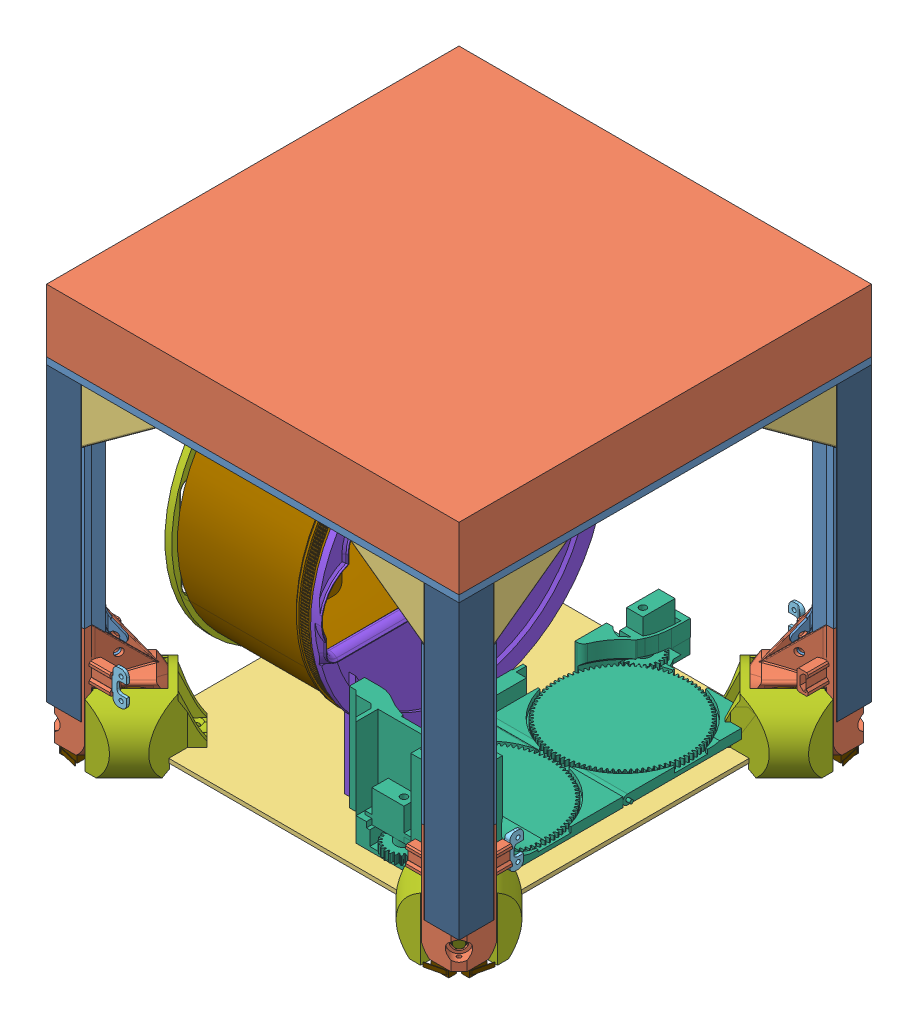
SolidWorks assembly MK7 IEEE BOT, configuration Default. Lengths in mm.
Overall size (425.24 302.29 425.24).
113 component instances, 29 part files, 44 mates.
Components (placement in the parent):
- MK5 Top Plate-1: MK5 Top Plate [Default] at (0 249 0) size (301.62 5 301.62)
- LEG assem MK5-1: LEG assem MK5 [Default] at (121.6905 25.4 121.6905) x (-0.707107 0 0.707107) z (-0.707107 0 -0.707107) size (113.86 301.29 113.86)
  - Omniwheel Mount-MK5-1: Omniwheel Mount-MK5 [Default] x (0 0 -1) z (1 0 0) size (67.69 82.93 55.08)
  - Leg Bracket MK5-1: Leg Bracket MK5 [Default] at (0 223.6 -41.1848) x (-0.707107 0 0.707107) z (-0.707107 0 -0.707107) size (80.51 40 80.51)
  - Omniwheel Hub-1: Omniwheel Hub [Default] at (0 0 13.95) x (-0.608761 -0.793353 0) z (0.793353 -0.608761 0) size (15.82 24.5 15.7)
  - TOF sensor mount-1: TOF sensor mount [Default] at (-9.5304 0 9.5304) x (0.707107 0 0.707107) z (-0.707107 0 0.707107) size (3.8 25 24.25)
  - Pinion Drive-1: Pinion Drive [Default] at (-0.7071 228.6 -26.6539) size (107.48 45 51.62)
  - Bottom Plate Bracket-1: Bottom Plate Bracket [Default] at (0 0 21.75) size (66.29 52.5 63.07)
  - Bearing Slider-1: Bearing Slider [Default] at (-0.7071 261.6 -26.6539) x (1 0 0) z (0 1 0) size (23.6 12.46 20)
  - 2in 14mm omniwheel-MK5-1: 2in 14mm omniwheel-MK5 [Default] at origin size (55.39 55.39 27.5)
  - Steel 90 degree MK5-1: Steel 90 degree MK5 [8982K151] at (0 120.65 -23.2243) x (-0.707107 0 -0.707107) z (0 1 0) size (25.4 25.4 213.6)
  - Nema17.step-2: Nema17.step [Default] at (22.8737 252.6 18.2122) x (0 -1 0) z (-1 0 0) size (42 57.7 46)
  - hex flange nut_am-2: hex flange nut_am [B18.2.2.4M - Hex flange nut, M6 x 1 --N] at (0 0 27.75) x (0.990831 -0.135106 0) z (0 0 1) size (14.2 14.2 6)
  - instrument ball bearing_68_am-4: instrument ball bearing_68_am [AFBMA 12.1.4.1 - 0070-14 - 12,SI,NC,12_68] at (0 0 -22.7198) x (0 0 1) z (-0.999767 0.021607 0) size (3.5 14 14)
  - 6mm G2T Pully Gear-1: 6mm G2T Pully Gear [Default] at (0 0 -9.25) x (0.996082 -0.088439 0) z (0.088439 0.996082 0) size (16 16 16)
  - 6mm G2T Pully Gear-2: 6mm G2T Pully Gear [Default] at (0 249.6 -30.45) x (-0.989152 0.146897 0) z (0.146897 0.989152 0) size (16 16 16)
  - Belt-1: Belt [Default] at (0 249.6 -23.35) x (-0.989152 0.146897 0) z (0 0 1) size (51.67 261.89 6)
  - instrument ball bearing_68_am-5: instrument ball bearing_68_am [AFBMA 12.1.4.1 - 0070-14 - 12,SI,NC,12_68] at (0 0 20) x (0 0 1) z (-0.999898 0.014309 0) size (3.5 14 14)
  - hex flange screw_am-1: hex flange screw_am [B18.2.3.4M - Hex flange screw, M5 x 0.8 x 35 --16N] at (0 0 -30.0698) x (0 0 1) z (-0.776229 0.630451 0) size (40.6 11.4 11.4)
  - hex flange screw_am-2: hex flange screw_am [B18.2.3.4M - Hex flange screw, M5 x 0.8 x 35 --16N] at (0 249.6 10.15) x (0 0 -1) z (-0.786653 -0.617395 0) size (40.6 11.4 11.4)
  - instrument ball bearing_68_am-6: instrument ball bearing_68_am [AFBMA 12.1.4.1 - 0070-14 - 12,SI,NC,12_68] at (0 251.6 -10.2) x (0 0 1) z (-0.998037 -0.06263 0) size (3.5 14 14)
  - instrument ball bearing_68_am-7: instrument ball bearing_68_am [AFBMA 12.1.4.1 - 0070-14 - 12,SI,NC,12_68] at (0 251.6 -2.2359) x (0 0 1) z (-0.682316 -0.731058 0) size (3.5 14 14)
  - hex screw_am-1: hex screw_am [B18.6.7M - M4 x 0.7 x 40 Indented HHMS --40N] at (5 274.6 -7.2179) x (0 -1 0) z (0 0 1) size (43 8.08 7)
  - Microswitch-1: Microswitch [Default] at (5.7276 -18.7296 -25.8406) x (0.707107 0 0.707107) z (-0.707107 0 0.707107) size (15.16 5.8 14.13)
  - Microswitch-2: Microswitch [Default] at (-5.7276 -12.9296 -25.8406) x (-0.707107 0 0.707107) z (0.707107 0 0.707107) size (15.16 5.8 14.13)
  - BeltShroud-1: BeltShroud [Default] at (0 70 0) x (0 0 -1) z (0 1 0) size (24.44 39.03 180.07)
- LEG assem MK5-2: LEG assem MK5 [Default] at (121.6905 25.4 -121.6905) x (0.707107 0 0.707107) z (-0.707107 0 0.707107) size (113.86 301.29 113.86)
  - Omniwheel Mount-MK5-1: Omniwheel Mount-MK5 [Default] x (0 0 -1) z (1 0 0) size (67.69 82.93 55.08)
  - Leg Bracket MK5-1: Leg Bracket MK5 [Default] at (0 223.6 -41.1848) x (-0.707107 0 0.707107) z (-0.707107 0 -0.707107) size (80.51 40 80.51)
  - Omniwheel Hub-1: Omniwheel Hub [Default] at (0 0 13.95) x (-0.608761 -0.793353 0) z (0.793353 -0.608761 0) size (15.82 24.5 15.7)
  - TOF sensor mount-1: TOF sensor mount [Default] at (-9.5304 0 9.5304) x (0.707107 0 0.707107) z (-0.707107 0 0.707107) size (3.8 25 24.25)
  - Pinion Drive-1: Pinion Drive [Default] at (-0.7071 228.6 -26.6539) size (107.48 45 51.62)
  - Bottom Plate Bracket-1: Bottom Plate Bracket [Default] at (0 0 21.75) size (66.29 52.5 63.07)
  - Bearing Slider-1: Bearing Slider [Default] at (-0.7071 261.6 -26.6539) x (1 0 0) z (0 1 0) size (23.6 12.46 20)
  - 2in 14mm omniwheel-MK5-1: 2in 14mm omniwheel-MK5 [Default] at origin size (55.39 55.39 27.5)
  - Steel 90 degree MK5-1: Steel 90 degree MK5 [8982K151] at (0 120.65 -23.2243) x (-0.707107 0 -0.707107) z (0 1 0) size (25.4 25.4 213.6)
  - Nema17.step-2: Nema17.step [Default] at (22.8737 252.6 18.2122) x (0 -1 0) z (-1 0 0) size (42 57.7 46)
  - hex flange nut_am-2: hex flange nut_am [B18.2.2.4M - Hex flange nut, M6 x 1 --N] at (0 0 27.75) x (0.990831 -0.135106 0) z (0 0 1) size (14.2 14.2 6)
  - instrument ball bearing_68_am-4: instrument ball bearing_68_am [AFBMA 12.1.4.1 - 0070-14 - 12,SI,NC,12_68] at (0 0 -22.7198) x (0 0 1) z (-0.999767 0.021607 0) size (3.5 14 14)
  - 6mm G2T Pully Gear-1: 6mm G2T Pully Gear [Default] at (0 0 -9.25) x (0.996082 -0.088439 0) z (0.088439 0.996082 0) size (16 16 16)
  - 6mm G2T Pully Gear-2: 6mm G2T Pully Gear [Default] at (0 249.6 -30.45) x (-0.989152 0.146897 0) z (0.146897 0.989152 0) size (16 16 16)
  - Belt-1: Belt [Default] at (0 249.6 -23.35) x (-0.989152 0.146897 0) z (0 0 1) size (51.67 261.89 6)
  - instrument ball bearing_68_am-5: instrument ball bearing_68_am [AFBMA 12.1.4.1 - 0070-14 - 12,SI,NC,12_68] at (0 0 20) x (0 0 1) z (-0.999898 0.014309 0) size (3.5 14 14)
  - hex flange screw_am-1: hex flange screw_am [B18.2.3.4M - Hex flange screw, M5 x 0.8 x 35 --16N] at (0 0 -30.0698) x (0 0 1) z (-0.776229 0.630451 0) size (40.6 11.4 11.4)
  - hex flange screw_am-2: hex flange screw_am [B18.2.3.4M - Hex flange screw, M5 x 0.8 x 35 --16N] at (0 249.6 10.15) x (0 0 -1) z (-0.786653 -0.617395 0) size (40.6 11.4 11.4)
  - instrument ball bearing_68_am-6: instrument ball bearing_68_am [AFBMA 12.1.4.1 - 0070-14 - 12,SI,NC,12_68] at (0 251.6 -10.2) x (0 0 1) z (-0.998037 -0.06263 0) size (3.5 14 14)
  - instrument ball bearing_68_am-7: instrument ball bearing_68_am [AFBMA 12.1.4.1 - 0070-14 - 12,SI,NC,12_68] at (0 251.6 -2.2359) x (0 0 1) z (-0.682316 -0.731058 0) size (3.5 14 14)
  - hex screw_am-1: hex screw_am [B18.6.7M - M4 x 0.7 x 40 Indented HHMS --40N] at (5 274.6 -7.2179) x (0 -1 0) z (0 0 1) size (43 8.08 7)
  - Microswitch-1: Microswitch [Default] at (5.7276 -18.7296 -25.8406) x (0.707107 0 0.707107) z (-0.707107 0 0.707107) size (15.16 5.8 14.13)
  - Microswitch-2: Microswitch [Default] at (-5.7276 -12.9296 -25.8406) x (-0.707107 0 0.707107) z (0.707107 0 0.707107) size (15.16 5.8 14.13)
  - BeltShroud-1: BeltShroud [Default] at (0 70 0) x (0 0 -1) z (0 1 0) size (24.44 39.03 180.07)
- LEG assem MK5-3: LEG assem MK5 [Default] at (-121.6905 25.4 -121.6905) x (0.707107 0 -0.707107) z (0.707107 0 0.707107) size (113.86 301.29 113.86)
  - Omniwheel Mount-MK5-1: Omniwheel Mount-MK5 [Default] x (0 0 -1) z (1 0 0) size (67.69 82.93 55.08)
  - Leg Bracket MK5-1: Leg Bracket MK5 [Default] at (0 223.6 -41.1848) x (-0.707107 0 0.707107) z (-0.707107 0 -0.707107) size (80.51 40 80.51)
  - Omniwheel Hub-1: Omniwheel Hub [Default] at (0 0 13.95) x (-0.608761 -0.793353 0) z (0.793353 -0.608761 0) size (15.82 24.5 15.7)
  - TOF sensor mount-1: TOF sensor mount [Default] at (-9.5304 0 9.5304) x (0.707107 0 0.707107) z (-0.707107 0 0.707107) size (3.8 25 24.25)
  - Pinion Drive-1: Pinion Drive [Default] at (-0.7071 228.6 -26.6539) size (107.48 45 51.62)
  - Bottom Plate Bracket-1: Bottom Plate Bracket [Default] at (0 0 21.75) size (66.29 52.5 63.07)
  - Bearing Slider-1: Bearing Slider [Default] at (-0.7071 261.6 -26.6539) x (1 0 0) z (0 1 0) size (23.6 12.46 20)
  - 2in 14mm omniwheel-MK5-1: 2in 14mm omniwheel-MK5 [Default] at origin size (55.39 55.39 27.5)
  - Steel 90 degree MK5-1: Steel 90 degree MK5 [8982K151] at (0 120.65 -23.2243) x (-0.707107 0 -0.707107) z (0 1 0) size (25.4 25.4 213.6)
  - Nema17.step-2: Nema17.step [Default] at (22.8737 252.6 18.2122) x (0 -1 0) z (-1 0 0) size (42 57.7 46)
  - hex flange nut_am-2: hex flange nut_am [B18.2.2.4M - Hex flange nut, M6 x 1 --N] at (0 0 27.75) x (0.990831 -0.135106 0) z (0 0 1) size (14.2 14.2 6)
  - instrument ball bearing_68_am-4: instrument ball bearing_68_am [AFBMA 12.1.4.1 - 0070-14 - 12,SI,NC,12_68] at (0 0 -22.7198) x (0 0 1) z (-0.999767 0.021607 0) size (3.5 14 14)
  - 6mm G2T Pully Gear-1: 6mm G2T Pully Gear [Default] at (0 0 -9.25) x (0.996082 -0.088439 0) z (0.088439 0.996082 0) size (16 16 16)
  - 6mm G2T Pully Gear-2: 6mm G2T Pully Gear [Default] at (0 249.6 -30.45) x (-0.989152 0.146897 0) z (0.146897 0.989152 0) size (16 16 16)
  - Belt-1: Belt [Default] at (0 249.6 -23.35) x (-0.989152 0.146897 0) z (0 0 1) size (51.67 261.89 6)
  - instrument ball bearing_68_am-5: instrument ball bearing_68_am [AFBMA 12.1.4.1 - 0070-14 - 12,SI,NC,12_68] at (0 0 20) x (0 0 1) z (-0.999898 0.014309 0) size (3.5 14 14)
  - hex flange screw_am-1: hex flange screw_am [B18.2.3.4M - Hex flange screw, M5 x 0.8 x 35 --16N] at (0 0 -30.0698) x (0 0 1) z (-0.776229 0.630451 0) size (40.6 11.4 11.4)
  - hex flange screw_am-2: hex flange screw_am [B18.2.3.4M - Hex flange screw, M5 x 0.8 x 35 --16N] at (0 249.6 10.15) x (0 0 -1) z (-0.786653 -0.617395 0) size (40.6 11.4 11.4)
  - instrument ball bearing_68_am-6: instrument ball bearing_68_am [AFBMA 12.1.4.1 - 0070-14 - 12,SI,NC,12_68] at (0 251.6 -10.2) x (0 0 1) z (-0.998037 -0.06263 0) size (3.5 14 14)
  - instrument ball bearing_68_am-7: instrument ball bearing_68_am [AFBMA 12.1.4.1 - 0070-14 - 12,SI,NC,12_68] at (0 251.6 -2.2359) x (0 0 1) z (-0.682316 -0.731058 0) size (3.5 14 14)
  - hex screw_am-1: hex screw_am [B18.6.7M - M4 x 0.7 x 40 Indented HHMS --40N] at (5 274.6 -7.2179) x (0 -1 0) z (0 0 1) size (43 8.08 7)
  - Microswitch-1: Microswitch [Default] at (5.7276 -18.7296 -25.8406) x (0.707107 0 0.707107) z (-0.707107 0 0.707107) size (15.16 5.8 14.13)
  - Microswitch-2: Microswitch [Default] at (-5.7276 -12.9296 -25.8406) x (-0.707107 0 0.707107) z (0.707107 0 0.707107) size (15.16 5.8 14.13)
  - BeltShroud-1: BeltShroud [Default] at (0 70 0) x (0 0 -1) z (0 1 0) size (24.44 39.03 180.07)
- LEG assem MK5-4: LEG assem MK5 [Default] at (-121.6905 25.4 121.6905) x (-0.707107 0 -0.707107) z (0.707107 0 -0.707107) size (113.86 301.29 113.86)
  - Omniwheel Mount-MK5-1: Omniwheel Mount-MK5 [Default] x (0 0 -1) z (1 0 0) size (67.69 82.93 55.08)
  - Leg Bracket MK5-1: Leg Bracket MK5 [Default] at (0 223.6 -41.1848) x (-0.707107 0 0.707107) z (-0.707107 0 -0.707107) size (80.51 40 80.51)
  - Omniwheel Hub-1: Omniwheel Hub [Default] at (0 0 13.95) x (-0.608761 -0.793353 0) z (0.793353 -0.608761 0) size (15.82 24.5 15.7)
  - TOF sensor mount-1: TOF sensor mount [Default] at (-9.5304 0 9.5304) x (0.707107 0 0.707107) z (-0.707107 0 0.707107) size (3.8 25 24.25)
  - Pinion Drive-1: Pinion Drive [Default] at (-0.7071 228.6 -26.6539) size (107.48 45 51.62)
  - Bottom Plate Bracket-1: Bottom Plate Bracket [Default] at (0 0 21.75) size (66.29 52.5 63.07)
  - Bearing Slider-1: Bearing Slider [Default] at (-0.7071 261.6 -26.6539) x (1 0 0) z (0 1 0) size (23.6 12.46 20)
  - 2in 14mm omniwheel-MK5-1: 2in 14mm omniwheel-MK5 [Default] at origin size (55.39 55.39 27.5)
  - Steel 90 degree MK5-1: Steel 90 degree MK5 [8982K151] at (0 120.65 -23.2243) x (-0.707107 0 -0.707107) z (0 1 0) size (25.4 25.4 213.6)
  - Nema17.step-2: Nema17.step [Default] at (22.8737 252.6 18.2122) x (0 -1 0) z (-1 0 0) size (42 57.7 46)
  - hex flange nut_am-2: hex flange nut_am [B18.2.2.4M - Hex flange nut, M6 x 1 --N] at (0 0 27.75) x (0.990831 -0.135106 0) z (0 0 1) size (14.2 14.2 6)
  - instrument ball bearing_68_am-4: instrument ball bearing_68_am [AFBMA 12.1.4.1 - 0070-14 - 12,SI,NC,12_68] at (0 0 -22.7198) x (0 0 1) z (-0.999767 0.021607 0) size (3.5 14 14)
  - 6mm G2T Pully Gear-1: 6mm G2T Pully Gear [Default] at (0 0 -9.25) x (0.996082 -0.088439 0) z (0.088439 0.996082 0) size (16 16 16)
  - 6mm G2T Pully Gear-2: 6mm G2T Pully Gear [Default] at (0 249.6 -30.45) x (-0.989152 0.146897 0) z (0.146897 0.989152 0) size (16 16 16)
  - Belt-1: Belt [Default] at (0 249.6 -23.35) x (-0.989152 0.146897 0) z (0 0 1) size (51.67 261.89 6)
  - instrument ball bearing_68_am-5: instrument ball bearing_68_am [AFBMA 12.1.4.1 - 0070-14 - 12,SI,NC,12_68] at (0 0 20) x (0 0 1) z (-0.999898 0.014309 0) size (3.5 14 14)
  - hex flange screw_am-1: hex flange screw_am [B18.2.3.4M - Hex flange screw, M5 x 0.8 x 35 --16N] at (0 0 -30.0698) x (0 0 1) z (-0.776229 0.630451 0) size (40.6 11.4 11.4)
  - hex flange screw_am-2: hex flange screw_am [B18.2.3.4M - Hex flange screw, M5 x 0.8 x 35 --16N] at (0 249.6 10.15) x (0 0 -1) z (-0.786653 -0.617395 0) size (40.6 11.4 11.4)
  - instrument ball bearing_68_am-6: instrument ball bearing_68_am [AFBMA 12.1.4.1 - 0070-14 - 12,SI,NC,12_68] at (0 251.6 -10.2) x (0 0 1) z (-0.998037 -0.06263 0) size (3.5 14 14)
  - instrument ball bearing_68_am-7: instrument ball bearing_68_am [AFBMA 12.1.4.1 - 0070-14 - 12,SI,NC,12_68] at (0 251.6 -2.2359) x (0 0 1) z (-0.682316 -0.731058 0) size (3.5 14 14)
  - hex screw_am-1: hex screw_am [B18.6.7M - M4 x 0.7 x 40 Indented HHMS --40N] at (5 274.6 -7.2179) x (0 -1 0) z (0 0 1) size (43 8.08 7)
  - Microswitch-1: Microswitch [Default] at (5.7276 -18.7296 -25.8406) x (0.707107 0 0.707107) z (-0.707107 0 0.707107) size (15.16 5.8 14.13)
  - Microswitch-2: Microswitch [Default] at (-5.7276 -12.9296 -25.8406) x (-0.707107 0 0.707107) z (0.707107 0 0.707107) size (15.16 5.8 14.13)
  - BeltShroud-1: BeltShroud [Default] at (0 70 0) x (0 0 -1) z (0 1 0) size (24.44 39.03 180.07)
- Leg Bracket MK5-1: Leg Bracket MK5 [Default] at (-150.8125 249 150.8125) size (80.51 40 80.51)
- Bottom Plate Bracket-1: Bottom Plate Bracket [Default] at (106.3109 25.4 -106.3109) x (0.707107 0 0.707107) z (-0.707107 0 0.707107) size (66.29 52.5 63.07)
- TopCover-1: TopCover [Default] at (0 254 0) x (1 0 0) z (0 1 0) size (301.63 301.63 46)
- Bottom Plate21-1: Bottom Plate21 [Default] at (-75.998 15.4 -153.7106) x (-0.707107 0 0.707107) z (0 -1 0) size (300.69 300.69 3)
- Nema14Pancake Stepper-1: Nema14Pancake Stepper [Default] at (-22.1225 272 0) x (0 0 -1) z (0 1 0) size (51 23.8 36)
- 3764N114_High-Strength Gt Timing Belt Pulley-1: 3764N114_High-Strength Gt Timing Belt Pulley [3764N114] at (-20.5438 272 0) x (0 -0.930392 -0.366566) z (-1 0 0) size (30.73 30.73 9.91)
- EleFlipAss.step-2: EleFlipAss.step [Default] at (32.351 21.5649 -11.7055) x (1 0 0) z (0 1 0) size (148 245.19 83.5)
- DrumHolderBackPlate.step-1: DrumHolderBackPlate.step [Default] at (-105.0625 135.4 0) x (0 0 1) z (-1 0 0) size (210 233.1 15.65)
- twist_inside_plate-2: twist_inside_plate [Default] at (-3.5625 135.4 0) size (8.95 233.6 210)
- StorageDrum3-1: StorageDrum3 [Default] at (-104.0625 135.4 0) x (0 0.402863 -0.91526) z (1 0 0) size (208.49 208.49 100.03)
- Part2^MK7 IEEE BOT-1: Part2^MK7 IEEE BOT [Default] at origin (virtual)
- NylonBushing-1: NylonBushing [Default] at (-104.8625 135.4 0) x (0 0.017134 0.999853) z (-1 0 0) size (30 30 1)
Mates (geometry in assembly coordinates):
- Coincident1: coincident aligned: plane of MK5 Top Plate-1 through (0 249 0) normal (0 0 1)
- Coincident2: coincident aligned: plane of MK5 Top Plate-1 through (0 249 0) normal (1 0 0)
- Distance1: distance = 254 mm aligned: plane of MK5 Top Plate-1 through (0 254 0) normal (0 1 0)
- Coincident3: coincident aligned: plane of MK5 Top Plate-1 through (-150.8125 254 150.8125) normal (0 0 1); plane of LEG assem MK5-1/Steel 90 degree MK5-1 through (125.4125 298.45 150.8125) normal (0 0 1)
- Coincident5: coincident aligned: plane of MK5 Top Plate-1 through (150.8125 254 150.8125) normal (1 0 0); plane of LEG assem MK5-1/Steel 90 degree MK5-1 through (150.8125 298.45 150.8125) normal (1 0 0)
- Coincident6: coincident aligned: plane of LEG assem MK5-1 through (121.6905 0 121.6905) normal (0 1 0)
- Coincident11: coincident aligned: plane of MK5 Top Plate-1 through (-150.8125 254 -150.8125) normal (0 0 -1); plane of LEG assem MK5-2/Steel 90 degree MK5-1 through (150.8125 298.45 -150.8125) normal (0 0 -1)
- Coincident12: coincident aligned: plane of MK5 Top Plate-1 through (150.8125 254 150.8125) normal (1 0 0); plane of LEG assem MK5-2/Steel 90 degree MK5-1 through (150.8125 298.45 -125.4125) normal (1 0 0)
- Coincident14: coincident aligned: plane of LEG assem MK5-2/Steel 90 degree MK5-1 through (150.8125 298.45 -150.8125) normal (0 0 -1); plane of LEG assem MK5-3/Steel 90 degree MK5-1 through (-125.4125 298.45 -150.8125) normal (0 0 -1)
- Coincident15: coincident aligned: plane of MK5 Top Plate-1 through (-150.8125 254 150.8125) normal (-1 0 0); plane of LEG assem MK5-3/Steel 90 degree MK5-1 through (-150.8125 298.45 -150.8125) normal (-1 0 0)
- Coincident17: coincident aligned: plane of MK5 Top Plate-1 through (-150.8125 254 150.8125) normal (-1 0 0); plane of LEG assem MK5-4/Steel 90 degree MK5-1 through (-150.8125 298.45 125.4125) normal (-1 0 0)
- Coincident18: coincident aligned: plane of MK5 Top Plate-1 through (-150.8125 254 150.8125) normal (0 0 1); plane of LEG assem MK5-4/Steel 90 degree MK5-1 through (-150.8125 298.45 150.8125) normal (0 0 1)
- Coincident29: coincident aligned: plane of MK5 Top Plate-1 through (-150.8125 254 150.8125) normal (0 0 1); plane of Leg Bracket MK5-1 through (-150.8125 249 150.8125) normal (0 0 1)
- Coincident30: coincident anti-aligned: plane of LEG assem MK5-4/Steel 90 degree MK5-1 through (-150.8125 298.45 125.4125) normal (-1 0 0); plane of Leg Bracket MK5-1 through (-150.8125 249 150.8125) normal (1 0 0)
- Coincident31: coincident anti-aligned: plane of MK5 Top Plate-1 through (0 249 0) normal (0 -1 0); plane of Leg Bracket MK5-1 through (-150.8125 249 150.8125) normal (0 1 0)
- Tangent1: tangent anti-aligned: plane of MK5 Top Plate-1 through (0 254 0) normal (0 1 0); cylinder of Nema14Pancake Stepper-1 through (-24.6225 272 0) axis (1 0 0) radius 18
- Coincident49: coincident: line of Nema14Pancake Stepper-1 through (-15.3225 272 0) axis (-1 0 0)
- Parallel2: parallel aligned: plane of MK5 Top Plate-1 through (0 254 0) normal (0 1 0); plane of Nema14Pancake Stepper-1 through (-22.1225 272 0) normal (0 1 0)
- Concentric3: concentric aligned: cylinder of Nema14Pancake Stepper-1 through (-15.3225 272 0) axis (-1 0 0) radius 2.5; cylinder of 3764N114_High-Strength Gt Timing Belt Pulley-1 through (-29.6751 272 0) axis (-1 0 0) radius 15.367
- Coincident50: coincident anti-aligned: plane of Nema14Pancake Stepper-1 through (-15.3225 272 0) normal (1 0 0); plane of 3764N114_High-Strength Gt Timing Belt Pulley-1 through (-15.3225 270.5905 2.3366) normal (-1 0 0)
- Coincident56: coincident anti-aligned: plane of MK5 Top Plate-1 through (0 249 0) normal (0 -1 0); plane of LEG assem MK5-3/Leg Bracket MK5-1 through (-150.8125 249 -150.8125) normal (0 1 0)
- Coincident57: coincident anti-aligned: plane of MK5 Top Plate-1 through (0 249 0) normal (0 -1 0); plane of LEG assem MK5-4/Leg Bracket MK5-1 through (-150.8125 249 150.8125) normal (0 1 0)
- Coincident58: coincident anti-aligned: plane of MK5 Top Plate-1 through (0 249 0) normal (0 -1 0); plane of LEG assem MK5-2/Leg Bracket MK5-1 through (150.8125 249 -150.8125) normal (0 1 0)
- InPlace5: in place: plane of LEG assem MK5-2/Omniwheel Mount-MK5-1 through (106.3109 25.4 -106.3109) normal (-0.707107 0 0.707107); plane of ? through (106.3109 0 -106.3109) normal (-0.707107 0 0.707107); moOrthogonalPlaneRef_w of LEG assem MK5-2/Omniwheel Mount-MK5-1 through (106.3109 25.4 -106.3109) normal (-0.707107 0 0.707107); plane of ? through (106.3109 0 -106.3109) normal (0 1 0); plane of LEG assem MK5-2/Omniwheel Mount-MK5-1 through (106.3109 25.4 -106.3109) normal (-0.707107 0 0.707107); plane of ? through (106.3109 0 -106.3109) normal (0.707107 0 0.707107); plane of LEG assem MK5-2/Omniwheel Mount-MK5-1 through (106.3109 25.4 -106.3109) normal (-0.707107 0 0.707107); unknown of ?
- Coincident59: coincident aligned: plane of LEG assem MK5-2/Omniwheel Mount-MK5-1; plane of Bottom Plate Bracket-1
- Coincident60: coincident aligned: moOrthogonalPlaneRef_w of LEG assem MK5-2/Omniwheel Mount-MK5-1 through (106.3109 25.4 -106.3109) normal (0 1 0); plane of Bottom Plate Bracket-1 through (106.3109 25.4 -106.3109) normal (0 1 0)
- Coincident61: coincident anti-aligned: moOrthogonalPlaneRef_w of LEG assem MK5-2/Omniwheel Mount-MK5-1 through (106.3109 25.4 -106.3109) normal (-0.707107 0 -0.707107); plane of Bottom Plate Bracket-1 through (106.3109 25.4 -106.3109) normal (0.707107 0 0.707107)
- Coincident59: coincident aligned: circle of LEG assem MK5-4/Bottom Plate Bracket-1; cylinder of Bottom Plate21-1 through (-92.6454 12.4 99.4703) axis (0 1 0) radius 2.25
- Coincident60: coincident anti-aligned: plane of LEG assem MK5-4/Bottom Plate Bracket-1 through (-100.1237 15.4 112.4981) normal (0 -1 0); plane of Bottom Plate21-1 through (-75.998 15.4 -153.7106) normal (0 1 0)
- Concentric6: concentric aligned: cylinder of LEG assem MK5-2/Bottom Plate Bracket-1 through (99.4703 9.4 -92.6454) axis (0 1 0) radius 2.25; cylinder of Bottom Plate21-1 through (99.4703 12.4 -92.6454) axis (0 1 0) radius 2.25
- InPlace6: in place: plane of MK5 Top Plate-1 through (0 254 0) normal (0 1 0); plane of TopCover-1 through (0 254 0) normal (0 1 0); plane of MK5 Top Plate-1 through (0 254 0) normal (0 1 0); plane of TopCover-1 through (0 254 0) normal (0 0 -1); plane of MK5 Top Plate-1 through (0 254 0) normal (0 1 0); plane of TopCover-1 through (0 254 0) normal (1 0 0); plane of MK5 Top Plate-1 through (0 254 0) normal (0 1 0); unknown of TopCover-1
- Coincident63: coincident aligned: plane of MK5 Top Plate-1; plane of ?
- Coincident64: coincident aligned: moOrthogonalPlaneRef_w of MK5 Top Plate-1 through (0 254 0) normal (0 0 -1); plane of TopCover-1 through (0 254 0) normal (0 0 -1)
- Coincident65: coincident anti-aligned: moOrthogonalPlaneRef_w of MK5 Top Plate-1 through (0 254 0) normal (-1 0 0); plane of TopCover-1 through (0 254 0) normal (1 0 0)
- Coincident62: coincident aligned: plane of DrumHolderBackPlate.step-1 through (-105.0625 135.4 0) normal (0 0 1)
- Distance3: distance = 40.75 mm aligned: plane of DrumHolderBackPlate.step-1 through (-110.0625 135.4 0) normal (-1 0 0); plane of LEG assem MK5-3/Steel 90 degree MK5-1 through (-150.8125 298.45 -150.8125) normal (-1 0 0)
- Parallel3: parallel aligned: plane of LEG assem MK5-4/Steel 90 degree MK5-1 through (-150.8125 298.45 150.8125) normal (0 0 1); plane of LEG assem MK5-1/Steel 90 degree MK5-1 through (125.4125 298.45 150.8125) normal (0 0 1)
- Coincident68: coincident anti-aligned: plane of MK5 Top Plate-1 through (0 249 0) normal (0 -1 0); plane of DrumHolderBackPlate.step-1 through (-132.3125 249 79.2101) normal (0 1 0)
- Concentric10: concentric aligned: cylinder of twist_inside_plate-2 through (-0.5625 135.4 0) axis (-1 0 0) radius 4; cylinder of StorageDrum3-1 through (-4.0511 135.4 0) axis (-1 0 0) radius 5
- Distance4: distance = 1 mm anti-aligned: plane of StorageDrum3-1 through (-104.0625 135.4 0) normal (-1 0 0); plane of DrumHolderBackPlate.step-1 through (-105.0625 135.4 0) normal (1 0 0)
- Concentric11: concentric anti-aligned: cylinder of DrumHolderBackPlate.step-1 through (-108.0625 135.4 0) axis (1 0 0) radius 4.2; circle of NylonBushing-1
- Distance5: distance = 0.2 mm aligned: plane of DrumHolderBackPlate.step-1 through (-105.0625 135.4 0) normal (1 0 0); plane of NylonBushing-1 through (-104.8625 135.4 0) normal (1 0 0)
- Distance7: distance = 0.5 mm anti-aligned: plane of twist_inside_plate-2 through (-3.5625 135.4 0) normal (-1 0 0); plane of StorageDrum3-1 through (-4.0625 135.4 0) normal (1 0 0)
- Parallel4: parallel aligned: plane of Bottom Plate21-1 through (-75.998 15.4 -153.7106) normal (0 1 0); plane of twist_inside_plate-2 through (-110.5183 113.4 25.38) normal (0 1 0)
